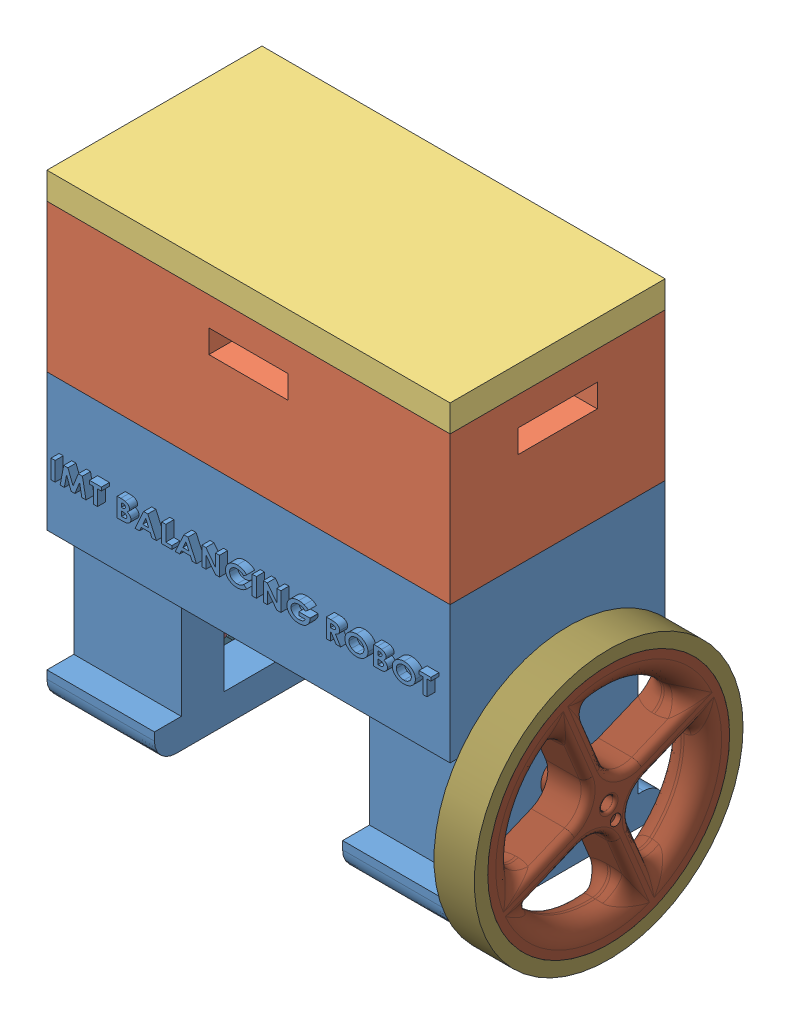
SolidWorks assembly Ensamblaje1, configuration Predeterminado. Lengths in mm.
Overall size (178.86 198.67 117.55).
21 component instances, 14 part files, 33 mates.
Components (placement in the parent):
- Pieza1-1: Pieza1 [Predeterminado] at (-28.3186 -30.7691 0) size (150 107 83)
- Pieza2-1: Pieza2 [Predeterminado] at (-28.3186 76.2309 0) size (150 62.5 80)
- Pieza4-1: Pieza4 [Predeterminado] at (-28.3186 131.2309 0) size (150 17.5 80)
- HiLetgo ESP32.STEP-1: HiLetgo ESP32.STEP [Predeterminado] at (10.1044 84.6129 5.87) x (-1 0 0) z (0 0 -1) size (25.65 13.21 49.13)
  - HiLetgo ESP32.STEP-1: HiLetgo ESP32.STEP [Predeterminado] at origin size (25.65 4.83 48.26)
  - molex_0473460001.STEP-1: molex_0473460001.STEP [Predeterminado] at (0 1.3434 -22.408) x (-1 0 0) z (0 0 -1) size (8.25 3.45 5.94)
  - PCB Button.STEP-1: PCB Button.STEP [Predeterminado] at (7.62 1.524 -21.463) size (2.79 1.27 3.81)
  - PCB Button.STEP-2: PCB Button.STEP [Predeterminado] at (-7.62 1.524 -21.463) x (-1 0 0) z (0 0 -1) size (2.79 1.27 3.81)
  - Pin Headers ESP32.STEP-1: Pin Headers ESP32.STEP [Predeterminado] at (11.557 -2.286 -5.334) size (2.29 11.18 48.26)
  - Pin Headers ESP32.STEP-2: Pin Headers ESP32.STEP [Predeterminado] at (-11.557 -2.286 -5.334) size (2.29 11.18 48.26)
- Pololu A4899.stp-1: Pololu A4899.stp [Predeterminado] at (-100.8147 72.5019 0.0075) x (0 0 -1) z (0 1 0) size (20.32 15.24 12.75)
- Pololu A4899.stp-2: Pololu A4899.stp [Predeterminado] at (-100.8147 72.5019 39.6875) x (0 0 -1) z (0 1 0) size (20.32 15.24 12.75)
- pololu.STEP-1: pololu.STEP [Predeterminado] at (-2.0619 81.6271 2.3344) x (0 0 1) z (-1 0 0) size (12.7 10 25.4)
  - Header5.STEP-1: Header5.STEP [Predeterminado] at (-7.3344 -1.8962 12.7) size (12.7 10 2.54)
  - Pol.STEP-1: Pol.STEP [Predeterminado] at (5.3656 2.8038 36.83) x (-1 0 0) z (0 0 1) size (12.7 2.02 25.4)
- rin-1: rin [Predeterminado] at (-122.3186 1.3309 0) x (0 -1 0) z (0 0 1) size (90 22.59 90) (hidden)
- rin-2: rin [Predeterminado] at (65.6814 1.3309 0) x (0 -0.381849 0.924225) z (0 -0.924225 -0.381849) size (90 22.59 90)
- goma-1: goma [Predeterminado] at (50.6814 1.3309 0) x (0 -1 0) z (0 0 1) size (100 15 100)
- goma-2: goma [Predeterminado] at (-107.3186 1.3309 0) x (0 -1 0) z (0 0 -1) size (100 15 100) (hidden)
- Pololu - 1_250 Micro gear motor-1: Pololu - 1_250 Micro gear motor [Default] at (-86.8186 -14.7691 0.15) x (0 0 -1) z (-1 0 0) size (12 10 35.27)
- Pololu Magnetic Encoder #1523-1: Pololu Magnetic Encoder #1523 [Défaut] at (-79.3186 -14.7691 0.15) x (0 0 1) z (1 0 0) size (20 16.5 1.5)
Mates (geometry in assembly coordinates):
- Concéntrica1: concentric aligned: cylinder of Pieza1-1 through (41.6814 1.3309 0) axis (1 0 0) radius 11.15; cylinder of MICROCON_stepper motor_NEMA 17_SX17-1005LQCEF.stp-1 through (42.4314 1.3309 0) axis (1 0 0) radius 11
- Paralelo1: parallel anti-aligned: plane of Pieza1-1 through (-331.7268 25.2309 30) normal (0 -1 0); plane of MICROCON_stepper motor_NEMA 17_SX17-1005LQCEF.stp-1 through (11.4814 22.4809 -16.5409) normal (0 1 0)
- Coincidente5: coincident anti-aligned: plane of Pieza1-1 through (41.6814 -30.7691 0) normal (-1 0 0); plane of MICROCON_stepper motor_NEMA 17_SX17-1005LQCEF.stp-1 through (41.6814 1.3309 0) normal (1 0 0)
- Coincidente6: coincident anti-aligned: plane of Pieza1-1 through (-93.3186 76.2309 0) normal (1 0 0); plane of Pieza2-1 through (-93.3186 68.7309 0) normal (-1 0 0)
- Coincidente7: coincident anti-aligned: plane of Pieza1-1 through (-28.3186 76.2309 30) normal (0 0 -1); plane of Pieza2-1 through (-28.3186 68.7309 30) normal (0 0 1)
- Coincidente8: coincident anti-aligned: plane of Pieza1-1 through (-28.3186 76.2309 0) normal (0 1 0); plane of Pieza2-1 through (-28.3186 76.2309 0) normal (0 -1 0)
- Concéntrica2: concentric anti-aligned: cylinder of MICROCON_stepper motor_NEMA 17_SX17-1005LQCEF.stp-2 through (-91.9686 1.3309 0) axis (1 0 0) radius 2.5; cylinder of Pieza3-2 through (-103.3186 1.3309 0) axis (-1 0 0) radius 22
- Coincidente9: coincident anti-aligned: plane of Pieza1-1 through (-103.3186 -28.7691 40) normal (-1 0 0); plane of Pieza3-2 through (-103.3186 1.3309 0) normal (1 0 0)
- Coincidente10: coincident anti-aligned: plane of Pieza1-1 through (46.6814 -28.7691 40) normal (1 0 0); plane of Pieza3-1 through (46.6814 1.3309 0) normal (-1 0 0)
- Concéntrica3: concentric aligned: cylinder of MICROCON_stepper motor_NEMA 17_SX17-1005LQCEF.stp-1 through (35.3314 1.3309 0) axis (-1 0 0) radius 2.5; circle of Pieza3-1
- Coincidente15: coincident anti-aligned: plane of Pieza4-1 through (-93.3186 123.7309 0) normal (-1 0 0); plane of Pieza2-1 through (-93.3186 131.2309 30) normal (1 0 0)
- Coincidente16: coincident anti-aligned: plane of Pieza2-1 through (36.6814 131.2309 30) normal (0 0 -1); plane of Pieza4-1 through (-28.3186 123.7309 30) normal (0 0 1)
- Coincidente17: coincident anti-aligned: plane of Pieza2-1 through (36.6814 131.2309 30) normal (0 0 -1); plane of HiLetgo ESP32.STEP-1/HiLetgo ESP32.STEP-1 through (22.9314 86.1369 30) normal (0 0 1)
- Coincidente19: coincident anti-aligned: plane of Pieza2-1 through (-28.3186 76.2309 0) normal (0 1 0); plane of HiLetgo ESP32.STEP-1/Pin Headers ESP32.STEP-2 through (21.6614 76.2309 3.584) normal (0 -1 0)
- Coincidente20: coincident anti-aligned: plane of Pieza2-1 through (-28.3186 76.2309 0) normal (0 1 0); plane of Pololu A4899.stp-1 through (-100.8147 76.2309 0.0075) normal (0 -1 0)
- Coincidente21: coincident anti-aligned: plane of Pieza2-1 through (-28.3186 76.2309 0) normal (0 1 0); plane of Pololu A4899.stp-2 through (-100.8147 76.2309 39.6875) normal (0 -1 0)
- Coincidente22: coincident anti-aligned: plane of Pieza2-1 through (36.6814 131.2309 30) normal (0 0 -1); plane of Pololu A4899.stp-2 through (-76.0469 82.2309 30) normal (0 0 1)
- Coincidente23: coincident anti-aligned: plane of Pieza2-1 through (36.6814 131.2309 -30) normal (0 0 1); plane of Pololu A4899.stp-1 through (-60.8069 82.2309 -30) normal (0 0 -1)
- Coincidente25: coincident aligned: plane of Pololu A4899.stp-1 through (-60.8069 82.2309 -30) normal (1 0 0); plane of Pololu A4899.stp-2 through (-60.8069 82.2309 9.68) normal (1 0 0)
- Coincidente26: coincident anti-aligned: plane of Pieza2-1 through (-28.3186 76.2309 0) normal (0 1 0); plane of pololu.STEP-1/Header5.STEP-1 through (-16.0319 76.2309 7.7) normal (0 -1 0)
- Distancia1: distance = 25 mm anti-aligned: plane of Pieza2-1 through (36.6814 131.2309 -30) normal (0 0 1); plane of pololu.STEP-1/Pol.STEP-1 through (-38.8919 83.2309 -5) normal (0 0 -1)
- Concéntrica4: concentric aligned: cylinder of MICROCON_stepper motor_NEMA 17_SX17-1005LQCEF.stp-1 through (35.3314 1.3309 0) axis (-1 0 0) radius 2.5; cylinder of rin-2 through (65.6814 1.3309 0) axis (-1 0 0) radius 2.495
- Coincidente27: coincident anti-aligned: plane of MICROCON_stepper motor_NEMA 17_SX17-1005LQCEF.stp-1 through (43.6814 1.3309 -4.9) normal (1 0 0); plane of rin-2 through (43.6814 1.3309 0) normal (-1 0 0)
- Coincidente28: coincident anti-aligned: plane of MICROCON_stepper motor_NEMA 17_SX17-1005LQCEF.stp-2 through (-100.3186 1.3309 4.9) normal (-1 0 0); plane of rin-1 through (-100.3186 1.3309 0) normal (1 0 0)
- Concéntrica5: concentric aligned: cylinder of MICROCON_stepper motor_NEMA 17_SX17-1005LQCEF.stp-2 through (-91.9686 1.3309 0) axis (1 0 0) radius 2.5; cylinder of rin-1 through (-122.3186 1.3309 0) axis (1 0 0) radius 2.495
- Concéntrica6: concentric anti-aligned: cylinder of rin-2 through (50.6814 1.3309 0) axis (1 0 0) radius 45; cylinder of goma-1 through (65.6814 1.3309 0) axis (-1 0 0) radius 42
- Coincidente29: coincident aligned: plane of rin-2 through (65.6814 1.3309 0) normal (1 0 0); plane of goma-1 through (65.6814 1.3309 0) normal (1 0 0)
- Coincidente30: coincident anti-aligned: plane of Pieza2-1 through (-28.3186 131.2309 0) normal (0 1 0); plane of Pieza4-1 through (-28.3186 131.2309 0) normal (0 -1 0)
- Coincidente31: coincident anti-aligned: plane of Pieza1-1 through (-103.3186 -19.7691 -6.15) normal (0 1 0); plane of Pololu - 1_250 Micro gear motor-1 through (-94.3186 -19.7691 -3.1666) normal (0 -1 0)
- Coincidente32: coincident aligned: plane of Pieza1-1 through (-103.3186 -28.7691 40) normal (-1 0 0); plane of Pololu - 1_250 Micro gear motor-1 through (-103.3186 -10.7691 5.15) normal (-1 0 0)
- Coincidente33: coincident anti-aligned: plane of Pieza1-1 through (-103.3186 -19.7691 6.15) normal (0 0 -1); plane of Pololu - 1_250 Micro gear motor-1 through (-102.3186 -10.7691 6.15) normal (0 0 1)
- Coincidente34: coincident: plane of Pololu - 1_250 Micro gear motor-1 through (-79.3186 -10.7691 -2.85) normal (1 0 0); plane of Pololu Magnetic Encoder #1523-1 through (-79.3186 -14.2691 1.3635) normal (-1 0 0)
- Concéntrica9: concentric aligned: cylinder of Pololu - 1_250 Micro gear motor-1 through (-77.8186 -14.7691 0.15) axis (-1 0 0) radius 2.5; cylinder of Pololu Magnetic Encoder #1523-1 through (-78.3186 -14.7691 0.15) axis (-1 0 0) radius 2.5
